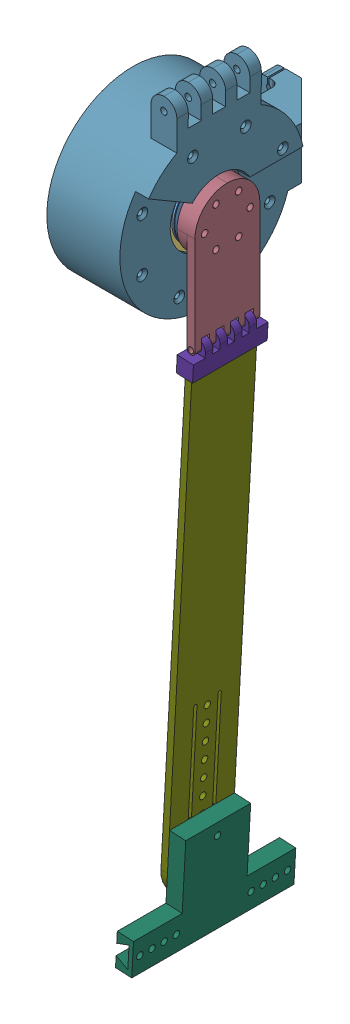
SolidWorks assembly ThighAssem_v1, configuration Default. Lengths in mm.
Overall size (60.96 456.03 136.26).
39 component instances, 23 part files, 9 mates.
Components (placement in the parent):
- BenchTestAssem-1: BenchTestAssem [Default] at (-13.4037 90.1362 110.0669) size (56.74 112 98)
  - TestingPaddle-1: TestingPaddle [Default] at (33.9401 55.0956 78.3658) x (0 -1 0) z (0 0 1) size (36.4 96 36.4) (hidden)
  - actuator_attach (1)-2: actuator_attach (1) [Default] at (120.9868 109.2347 94.0696) x (0 0 -1) z (-1 0 0) size (98 98 42.51)
    - 202011-ActPack-Geared.STEP-1: 202011-ActPack-Geared.STEP [Default] at (35.2154 51.7879 75.5049) size (98 98 42.51)
      - AK80-9 3D.STEP-1: AK80-9 3D.STEP [Default] at (0 -501.6085 -756.5855) x (0 0 1) z (-1 0 0) size (28.5 98 98)
        - AK80-9 3D(2)^AK80-9 3D.STEP-1: AK80-9 3D(2)^AK80-9 3D.STEP [Default] at origin size (28.5 98 98)
          - AK80-9_ASM_ASM^AK80-9 3D(2)_AK80-9 3D.STEP-1: AK80-9_ASM_ASM^AK80-9 3D(2)_AK80-9 3D.STEP [Default] at origin size (28.5 98 98)
            - PRODUCT_46766_ASM_ASM^AK80-9_ASM_ASM_AK80-9 3D(2)_AK80-9 3D.STEP-1: PRODUCT_46766_ASM_ASM^AK80-9_ASM_ASM_AK80-9 3D(2)_AK80-9 3D.STEP [Default] at origin size (28.5 98 98)
              - ____5^PRODUCT_46766_ASM_ASM_AK80-9_ASM_ASM_AK80-9 3D(2)_AK80-9 3D.STEP-1: ____5^PRODUCT_46766_ASM_ASM_AK80-9_ASM_ASM_AK80-9 3D(2)_AK80-9 3D.STEP [Default] at origin size (7.5 37 37)
              - ____1^PRODUCT_46766_ASM_ASM_AK80-9_ASM_ASM_AK80-9 3D(2)_AK80-9 3D.STEP-1: ____1^PRODUCT_46766_ASM_ASM_AK80-9_ASM_ASM_AK80-9 3D(2)_AK80-9 3D.STEP [Default] at origin size (2 14 14) (hidden)
              - ____2^PRODUCT_46766_ASM_ASM_AK80-9-MODIFIED-20201030.STEP-1: ____2^PRODUCT_46766_ASM_ASM_AK80-9-MODIFIED-20201030.STEP [Default] at origin size (6 98 98)
              - ____7^PRODUCT_46766_ASM_ASM_AK80-9_ASM_ASM_AK80-9 3D(2)_AK80-9 3D.STEP-1: ____7^PRODUCT_46766_ASM_ASM_AK80-9_ASM_ASM_AK80-9 3D(2)_AK80-9 3D.STEP [Default] at origin size (24.23 98 98)
      - RIGID_4_1_USB_0_1.STEP-1: RIGID_4_1_USB_0_1.STEP [Default] at (-43.9 -8.8349 6.09) x (0 -1 0) z (0 0 1) size (12.35 9.94 4.02)
        - RIGID_4_1_USB_0_1(2)^RIGID_4_1_USB_0_1.STEP-1: RIGID_4_1_USB_0_1(2)^RIGID_4_1_USB_0_1.STEP [Default] at origin size (12.35 9.94 4.02)
          - J1^RIGID_4_1_USB_0_1(2)_RIGID_4_1_USB_0_1.STEP-1: J1^RIGID_4_1_USB_0_1(2)_RIGID_4_1_USB_0_1.STEP [Default] at origin size (12.35 9.94 4.02)
            - CUI_DEVICES_UJ31-CH-3-MSMT-TR-67(2)^J1_RIGID_4_1_USB_0_1(2)_RIGID_4_1_USB_0_1.STEP-1: CUI_DEVICES_UJ31-CH-3-MSMT-TR-67(2)^J1_RIGID_4_1_USB_0_1(2)_RIGID_4_1_USB_0_1.STEP [Default] at (4.6001 0.25 0.31) x (0 1 0) z (1 0 0) size (9.94 4.02 12.35)
      - APL_P003_V41_MOUNTCOVER_MB.STEP-1: APL_P003_V41_MOUNTCOVER_MB.STEP [Default] at origin size (96 98 15.01)
      - APL_P004_V41_USBMOUNT_MB.STEP-1: APL_P004_V41_USBMOUNT_MB.STEP [Default] at (-47 22.0077 2.5) x (0 -1 0) z (0 0 1) size (44.02 7.7 7.3)
      - FX_P001_V41_RIGID_LUMP.STEP-1: FX_P001_V41_RIGID_LUMP.STEP [Default] at (-39.0889 -43.5 3.51) x (1 0 0) z (0 0 1) size (13.96 13.31 8.46)
      - PLP2-100.STEP-1: PLP2-100.STEP [Default] at (5.21 0 1.7962) size (3.3 3.3 3.26)
      - APL_P001_V41_MOUNT.STEP-1: APL_P001_V41_MOUNT.STEP [Default] at origin size (96 98 2.5)
      - APL_P002_V41_COVER.STEP-1: APL_P002_V41_COVER.STEP [Default] at origin size (96 98 12.52)
      - 90236A106_ METRIC ALLOY STEEL TORX FLAT HEAD SCREWS (1)_90236A106.STEP-1: 90236A106_ METRIC ALLOY STEEL TORX FLAT HEAD SCREWS (1)_90236A106.STEP [Default] at (-42.05 19.2577 11.1) size (3.8 3.8 0.9)
      - 90236A106_ METRIC ALLOY STEEL TORX FLAT HEAD SCREWS (1)_90236A106.STEP-2: 90236A106_ METRIC ALLOY STEEL TORX FLAT HEAD SCREWS (1)_90236A106.STEP [Default] at (-42.05 -19.2577 11.1) size (3.8 3.8 0.9)
      - 90910A920_LOW-PROFILE BUTTON HEAD TORX MACHINE SCREW (1)_90910A920.STEP-1: 90910A920_LOW-PROFILE BUTTON HEAD TORX MACHINE SCREW (1)_90910A920.STEP [Default] at (0 -46.25 5.5) size (3.8 3.8 1.1)
      - 90910A920_LOW-PROFILE BUTTON HEAD TORX MACHINE SCREW (1)_90910A920.STEP-2: 90910A920_LOW-PROFILE BUTTON HEAD TORX MACHINE SCREW (1)_90910A920.STEP [Default] at (42.05 -19.2577 5.5) x (0.987351 0.158553 0) z (0 0 1) size (3.8 3.8 1.1)
      - 90910A920_LOW-PROFILE BUTTON HEAD TORX MACHINE SCREW (1)_90910A920.STEP-3: 90910A920_LOW-PROFILE BUTTON HEAD TORX MACHINE SCREW (1)_90910A920.STEP [Default] at (42.05 19.2577 5.5) x (0.959125 0.282984 0) z (0 0 1) size (3.8 3.8 1.1)
      - 90910A920_LOW-PROFILE BUTTON HEAD TORX MACHINE SCREW (1)_90910A920.STEP-4: 90910A920_LOW-PROFILE BUTTON HEAD TORX MACHINE SCREW (1)_90910A920.STEP [Default] at (28 36.8112 5.5) x (0.928571 0.371154 0) z (0 0 1) size (3.8 3.8 1.1)
      - 90910A920_LOW-PROFILE BUTTON HEAD TORX MACHINE SCREW (1)_90910A920.STEP-5: 90910A920_LOW-PROFILE BUTTON HEAD TORX MACHINE SCREW (1)_90910A920.STEP [Default] at (-28 36.8112 5.5) x (0.906989 0.421154 0) z (0 0 1) size (3.8 3.8 1.1)
    - Hub_plate^actuator_attach (1)-1: Hub_plate^actuator_attach (1) [Default] at (35.2154 -449.8206 51.0049) x (-1 0 0) z (0 0 -1) size (98 98 5) (hidden, virtual)
    - Rotor_plate^actuator_attach (1)-1: Rotor_plate^actuator_attach (1) [Default] at (35.2154 -449.8206 48.0049) x (-1 0 0) z (0 0 -1) size (44 44 5) (hidden, virtual)
  - TestingPaddleCurve-2: TestingPaddleCurve [Default] at (129.9401 55.0956 78.3658) x (0 1 0) z (0 0 -1) size (54.8 56.01 20) (hidden)
  - 91290A172_BLACK-OXIDE CLASS 12.9 SOCKET HEAD CAP SCREW-2: 91290A172_BLACK-OXIDE CLASS 12.9 SOCKET HEAD CAP SCREW [91290A172] at (124.8152 56.3898 95.8238) size (7 7 34.44) (hidden)
  - RotorAttach_v1-1: RotorAttach_v1 [Default] at (76.2152 57.4467 58.8542) x (0 0 -1) z (1 0 0) size (40 83 11)
  - locking_mechanism2-1: locking_mechanism2 [Default] at (-70.6771 -140.5742 133.8857) x (0 0 -1) z (1 0 0)
- MotorHousingR_v2-1: MotorHousingR_v2 [Default] at (60.5782 147.583 168.9211) x (0 0.002091 0.999998) z (-1 0 0) size (136 125.5 53)
- ThighTShape_v1-1: ThighTShape_v1 [Default] at (63.5845 -175.6509 169.3211) x (0 0 -1) z (0.998473 -0.055247 0) size (100 60 12)
- ThighVertAdjust_v1-2: ThighVertAdjust_v1 [Default] at (54.1764 -218.9778 169.3211) x (0 0 1) z (-0.998473 0.055247 0) size (40 300 4)
- ThighHinge-1: ThighHinge [Default] at (71.1049 83.3487 169.1211) x (0 0 1) z (0.998473 -0.055247 0) size (46 18 10)
Mates (geometry in assembly coordinates):
- Coincident2: coincident anti-aligned: plane of BenchTestAssem-1/actuator_attach (1)-2/202011-ActPack-Geared.STEP-1/AK80-9 3D.STEP-1/AK80-9 3D(2)^AK80-9 3D.STEP-1/AK80-9_ASM_ASM^AK80-9 3D(2)_AK80-9 3D.STEP-1/PRODUCT_46766_ASM_ASM^AK80-9_ASM_ASM_AK80-9 3D(2)_AK80-9 3D.STEP-1/____7^PRODUCT_46766_ASM_ASM_AK80-9_ASM_ASM_AK80-9 3D(2)_AK80-9 3D.STEP-1 through (56.5782 123.583 168.9212) normal (1 0 0); plane of MotorHousingR_v2-1 through (56.5782 147.583 168.9211) normal (-1 0 0)
- Coincident5: coincident anti-aligned: plane of BenchTestAssem-1/RotorAttach_v1-1 through (73.8115 84.583 157.9211) normal (0 0 -1); plane of ThighHinge-1 through (66.5545 91.6127 157.9211) normal (0 0 1)
- Concentric1: concentric aligned: circle of BenchTestAssem-1/RotorAttach_v1-1; circle of ThighHinge-1
- Coincident6: coincident anti-aligned: plane of ThighVertAdjust_v1-2 through (70.7505 80.564 169.3211) normal (0.055247 0.998473 0); plane of ThighHinge-1 through (70.9502 80.5529 169.1211) normal (-0.055247 -0.998473 0)
- Coincident7: coincident anti-aligned: plane of ThighVertAdjust_v1-2 through (72.7475 80.4535 189.3211) normal (0 0 1); plane of ThighHinge-1 through (65.5601 73.6402 189.3211) normal (0 0 -1)
- Coincident8: coincident anti-aligned: plane of ThighVertAdjust_v1-2 through (68.7536 80.6745 149.3211) normal (-0.998473 0.055247 0); plane of ThighHinge-1 through (68.3558 73.4855 192.1211) normal (0.998473 -0.055247 0)
- Coincident10: coincident anti-aligned: plane of ThighTShape_v1-1 through (56.5952 -175.2642 160.8211) normal (0 0 -1); plane of ThighVertAdjust_v1-2 through (54.2364 -217.8938 160.8211) normal (0 0 1)
- Coincident11: coincident anti-aligned: plane of ThighTShape_v1-1 through (56.5952 -175.2642 169.3211) normal (-0.998473 0.055247 0); plane of ThighVertAdjust_v1-2 through (54.1764 -218.9778 169.3211) normal (0.998473 -0.055247 0)
- Concentric2: concentric anti-aligned: cylinder of BenchTestAssem-1/RotorAttach_v1-1 through (73.8115 147.583 168.9211) axis (-1 0 0) radius 20; cylinder of MotorHousingR_v2-1 through (21.5782 147.583 168.9211) axis (1 0 0) radius 22
